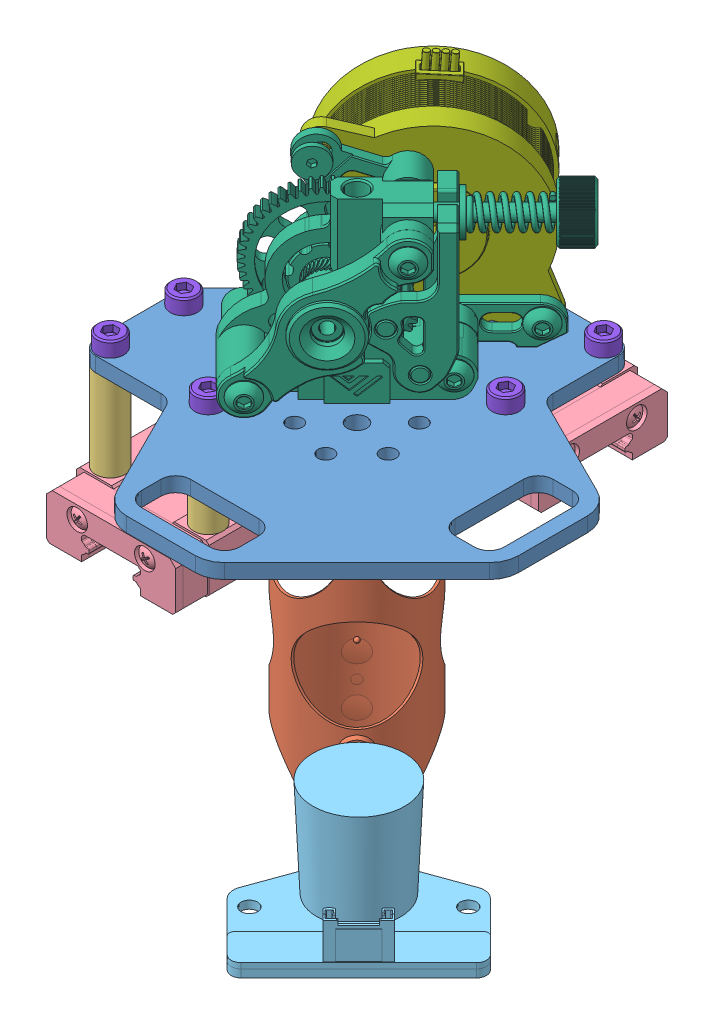
SolidWorks assembly ASM_Printhead_V1, configuration Default. Lengths in mm.
Overall size (87.58 123.94 98.13).
20 component instances, 8 part files, 39 mates.
Components (placement in the parent):
- PRT_Main_Plate_V1-1: PRT_Main_Plate_V1 [Default] at (19.5589 25.187 46.8985) size (81.5 3 81.5)
- PRT_Chube_Integration_V2-1: PRT_Chube_Integration_V2 [Default] at (-4.1383 -257.0883 22.8287) x (0.707107 0 -0.707107) z (0 1 0) size (26.81 27.92 66)
- PRT_M3x18_Standoff_V1-2: PRT_M3x18_Standoff_V1 [Default] at (-18.9411 7.187 58.7485) size (6 18 6)
- PRT_M3x18_Standoff_V1-3: PRT_M3x18_Standoff_V1 [Default] at (1.0589 7.187 58.7485) size (6 18 6)
- PRT_M3x18_Standoff_V1-4: PRT_M3x18_Standoff_V1 [Default] at (1.0589 7.187 43.7485) size (6 18 6)
- PRT_M3x18_Standoff_V1-5: PRT_M3x18_Standoff_V1 [Default] at (-18.9411 7.187 43.7485) size (6 18 6)
- PRT_MGN12C_Carriage-1: PRT_MGN12C_Carriage [Default] at (-8.9411 -0.313 51.2485) size (27 10 37.07)
- PRT_MGN12C_Carriage-2: PRT_MGN12C_Carriage [Default] at (23.9089 17.687 18.3985) x (0 0 -1) z (1 0 0) size (27 10 37.07)
- PRT_Beacon_RevH_Assm_Normal-1: PRT_Beacon_RevH_Assm_Normal [Default] at (38.27 -36.4022 65.237) x (0.707107 0 -0.707107) z (0 1 0) size (38 28.37 24.21)
- ASM_MA_Extruder_V1-1: ASM_MA_Extruder_V1 [Default] at (-20.6578 21.9691 29.4732) x (0.707107 0 -0.707107) z (0.707107 0 0.707107) size (62.49 57.22 45.42)
  - PRT_MA_VZ_Hextrudort-2: PRT_MA_VZ_Hextrudort [Default] at (16.116 12.2179 40.659) x (1 0 0) z (0 1 0) size (55.08 29 38.4)
  - PRT_MA_LDO_20mm_Nema14-1: PRT_MA_LDO_20mm_Nema14 [Default] at (-5.0462 48.6582 8.2878) x (-0.88148 0.472221 -0.000518) z (0.000441 -0.000274 -1) size (48.79 38.77 26.01)
- socket head cap screw_am-1: socket head cap screw_am [B18.3.1M - 3 x 0.5 x 25 Hex SHCS -- 18NHX] at (1.0589 31.187 58.7485) x (0 -1 0) z (0 0 1) size (28 5.5 5.5)
- socket head cap screw_am-2: socket head cap screw_am [B18.3.1M - 3 x 0.5 x 25 Hex SHCS -- 18NHX] at (-18.9411 31.187 58.7485) x (0 -1 0) z (0 0 1) size (28 5.5 5.5)
- socket head cap screw_am-3: socket head cap screw_am [B18.3.1M - 3 x 0.5 x 25 Hex SHCS -- 18NHX] at (-18.9411 31.187 43.7485) x (0 -1 0) z (0 0 1) size (28 5.5 5.5)
- socket head cap screw_am-4: socket head cap screw_am [B18.3.1M - 3 x 0.5 x 25 Hex SHCS -- 18NHX] at (1.0589 31.187 43.7485) x (0 -1 0) z (0 0 1) size (28 5.5 5.5)
- socket head cap screw_am-6: socket head cap screw_am [B18.3.1M - 3 x 0.5 x 6 Hex SHCS -- 6NHX] at (31.4089 31.187 8.3985) x (0 -1 0) z (0 0 1) size (9 5.5 5.5)
- socket head cap screw_am-7: socket head cap screw_am [B18.3.1M - 3 x 0.5 x 6 Hex SHCS -- 6NHX] at (31.4089 31.187 28.3985) x (0 -1 0) z (0 0 1) size (9 5.5 5.5)
- socket head cap screw_am-8: socket head cap screw_am [B18.3.1M - 3 x 0.5 x 6 Hex SHCS -- 6NHX] at (16.4089 31.187 28.3985) x (0 -1 0) z (0 0 1) size (9 5.5 5.5)
- socket head cap screw_am-9: socket head cap screw_am [B18.3.1M - 3 x 0.5 x 6 Hex SHCS -- 6NHX] at (16.4089 31.187 8.3985) x (0 -1 0) z (0 0 1) size (9 5.5 5.5)
Mates (geometry in assembly coordinates):
- Concentric1: concentric anti-aligned: cylinder of PRT_Main_Plate_V1-1 through (19.5589 28.187 46.8985) axis (0 1 0) radius 2; cylinder of PRT_Chube_Integration_V2-1 through (19.5589 25.187 46.8985) axis (0 -1 0) radius 2.05
- Coincident1: coincident anti-aligned: plane of PRT_Main_Plate_V1-1 through (19.5589 25.187 46.8985) normal (0 -1 0); plane of PRT_Chube_Integration_V2-1 through (22.0338 25.187 44.4236) normal (0 1 0)
- Concentric3: concentric anti-aligned: cylinder of PRT_Main_Plate_V1-1 through (13.195 28.187 53.2625) axis (0 1 0) radius 1.6; cylinder of PRT_Chube_Integration_V2-1 through (13.195 25.187 53.2625) axis (0 -1 0) radius 1.5
- Concentric41: concentric anti-aligned: cylinder of PRT_Main_Plate_V1-1 through (-18.9411 28.187 58.7485) axis (0 1 0) radius 1.6; cylinder of PRT_M3x18_Standoff_V1-2 through (-18.9411 25.187 58.7485) axis (0 -1 0) radius 3
- Coincident21: coincident anti-aligned: plane of PRT_Main_Plate_V1-1 through (19.5589 25.187 46.8985) normal (0 -1 0); plane of PRT_M3x18_Standoff_V1-2 through (-18.9411 25.187 58.7485) normal (0 1 0)
- Concentric51: concentric anti-aligned: cylinder of PRT_Main_Plate_V1-1 through (1.0589 28.187 58.7485) axis (0 1 0) radius 1.6; cylinder of PRT_M3x18_Standoff_V1-3 through (1.0589 25.187 58.7485) axis (0 -1 0) radius 3
- Coincident31: coincident anti-aligned: plane of PRT_Main_Plate_V1-1 through (19.5589 25.187 46.8985) normal (0 -1 0); plane of PRT_M3x18_Standoff_V1-3 through (1.0589 25.187 58.7485) normal (0 1 0)
- Concentric61: concentric anti-aligned: cylinder of PRT_Main_Plate_V1-1 through (1.0589 28.187 43.7485) axis (0 1 0) radius 1.6; cylinder of PRT_M3x18_Standoff_V1-4 through (1.0589 25.187 43.7485) axis (0 -1 0) radius 3
- Coincident41: coincident anti-aligned: plane of PRT_Main_Plate_V1-1 through (19.5589 25.187 46.8985) normal (0 -1 0); plane of PRT_M3x18_Standoff_V1-4 through (1.0589 25.187 43.7485) normal (0 1 0)
- Concentric71: concentric anti-aligned: cylinder of PRT_Main_Plate_V1-1 through (-18.9411 28.187 43.7485) axis (0 1 0) radius 1.6; cylinder of PRT_M3x18_Standoff_V1-5 through (-18.9411 25.187 43.7485) axis (0 -1 0) radius 3
- Coincident51: coincident anti-aligned: plane of PRT_Main_Plate_V1-1 through (19.5589 25.187 46.8985) normal (0 -1 0); plane of PRT_M3x18_Standoff_V1-5 through (-18.9411 25.187 43.7485) normal (0 1 0)
- Concentric8: concentric anti-aligned: cylinder of PRT_M3x18_Standoff_V1-4 through (1.0589 25.187 43.7485) axis (0 -1 0) radius 3; cylinder of PRT_MGN12C_Carriage-1 through (1.0589 7.187 43.7485) axis (0 1 0) radius 1.5
- Concentric9: concentric anti-aligned: cylinder of PRT_M3x18_Standoff_V1-2 through (-18.9411 25.187 58.7485) axis (0 -1 0) radius 3; cylinder of PRT_MGN12C_Carriage-1 through (-18.9411 7.187 58.7485) axis (0 1 0) radius 1.5
- Coincident6: coincident anti-aligned: plane of PRT_M3x18_Standoff_V1-2 through (-18.9411 7.187 58.7485) normal (0 -1 0); plane of PRT_MGN12C_Carriage-1 through (-15.3411 7.187 62.0985) normal (0 1 0)
- Concentric10: concentric aligned: cylinder of PRT_Main_Plate_V1-1 through (31.4089 28.187 28.3985) axis (0 1 0) radius 1.6; cylinder of PRT_MGN12C_Carriage-2 through (31.4089 25.187 28.3985) axis (0 1 0) radius 1.5
- Concentric11: concentric aligned: cylinder of PRT_Main_Plate_V1-1 through (16.4089 28.187 8.3985) axis (0 1 0) radius 1.6; cylinder of PRT_MGN12C_Carriage-2 through (16.4089 25.187 8.3985) axis (0 1 0) radius 1.5
- Coincident7: coincident anti-aligned: plane of PRT_Main_Plate_V1-1 through (19.5589 25.187 46.8985) normal (0 -1 0); plane of PRT_MGN12C_Carriage-2 through (34.7589 25.187 5.4985) normal (0 1 0)
- Concentric12: concentric aligned: cylinder of PRT_Main_Plate_V1-1 through (1.0589 28.187 58.7485) axis (0 1 0) radius 1.6; cylinder of socket head cap screw_am-1 through (1.0589 62.937 58.7485) axis (0 1 0) radius 2.75
- Coincident8: coincident anti-aligned: plane of PRT_Main_Plate_V1-1 through (19.5589 28.187 46.8985) normal (0 1 0); plane of socket head cap screw_am-1 through (3.8089 28.187 58.7485) normal (0 -1 0)
- Concentric13: concentric aligned: cylinder of PRT_Main_Plate_V1-1 through (-18.9411 28.187 58.7485) axis (0 1 0) radius 1.6; cylinder of socket head cap screw_am-2 through (-18.9411 62.937 58.7485) axis (0 1 0) radius 2.75
- Coincident9: coincident anti-aligned: plane of PRT_Main_Plate_V1-1 through (19.5589 28.187 46.8985) normal (0 1 0); plane of socket head cap screw_am-2 through (-16.1911 28.187 58.7485) normal (0 -1 0)
- Concentric14: concentric aligned: cylinder of PRT_Main_Plate_V1-1 through (-18.9411 28.187 43.7485) axis (0 1 0) radius 1.6; cylinder of socket head cap screw_am-3 through (-18.9411 62.937 43.7485) axis (0 1 0) radius 2.75
- Coincident10: coincident anti-aligned: plane of PRT_Main_Plate_V1-1 through (19.5589 28.187 46.8985) normal (0 1 0); plane of socket head cap screw_am-3 through (-16.1911 28.187 43.7485) normal (0 -1 0)
- Concentric15: concentric aligned: cylinder of PRT_Main_Plate_V1-1 through (1.0589 28.187 43.7485) axis (0 1 0) radius 1.6; cylinder of socket head cap screw_am-4 through (1.0589 62.937 43.7485) axis (0 1 0) radius 2.75
- Coincident11: coincident anti-aligned: plane of PRT_Main_Plate_V1-1 through (19.5589 28.187 46.8985) normal (0 1 0); plane of socket head cap screw_am-4 through (3.8089 28.187 43.7485) normal (0 -1 0)
- Concentric17: concentric aligned: cylinder of PRT_Main_Plate_V1-1 through (31.4089 28.187 8.3985) axis (0 1 0) radius 1.6; cylinder of socket head cap screw_am-6 through (31.4089 62.937 8.3985) axis (0 1 0) radius 2.75
- Coincident13: coincident anti-aligned: plane of PRT_Main_Plate_V1-1 through (19.5589 28.187 46.8985) normal (0 1 0); plane of socket head cap screw_am-6 through (34.1589 28.187 8.3985) normal (0 -1 0)
- Concentric18: concentric aligned: cylinder of PRT_Main_Plate_V1-1 through (31.4089 28.187 28.3985) axis (0 1 0) radius 1.6; cylinder of socket head cap screw_am-7 through (31.4089 62.937 28.3985) axis (0 1 0) radius 2.75
- Coincident14: coincident anti-aligned: plane of PRT_Main_Plate_V1-1 through (19.5589 28.187 46.8985) normal (0 1 0); plane of socket head cap screw_am-7 through (34.1589 28.187 28.3985) normal (0 -1 0)
- Concentric19: concentric aligned: cylinder of PRT_Main_Plate_V1-1 through (16.4089 28.187 28.3985) axis (0 1 0) radius 1.6; cylinder of socket head cap screw_am-8 through (16.4089 62.937 28.3985) axis (0 1 0) radius 2.75
- Coincident15: coincident anti-aligned: plane of PRT_Main_Plate_V1-1 through (19.5589 28.187 46.8985) normal (0 1 0); plane of socket head cap screw_am-8 through (19.1589 28.187 28.3985) normal (0 -1 0)
- Concentric20: concentric aligned: cylinder of PRT_Main_Plate_V1-1 through (16.4089 28.187 8.3985) axis (0 1 0) radius 1.6; cylinder of socket head cap screw_am-9 through (16.4089 62.937 8.3985) axis (0 1 0) radius 2.75
- Coincident16: coincident anti-aligned: plane of PRT_Main_Plate_V1-1 through (19.5589 28.187 46.8985) normal (0 1 0); plane of socket head cap screw_am-9 through (19.1589 28.187 8.3985) normal (0 -1 0)
- Distance2: distance = 4.8 mm aligned: plane of PRT_Beacon_RevH_Assm_Normal-1 through (38.27 -40.613 65.237) normal (0 -1 0); plane of PRT_Chube_Integration_V2-1 through (19.5589 -35.813 46.8985) normal (0 -1 0)
- Distance3: distance = 17.7 mm: point of PRT_Beacon_RevH_Assm_Normal-1; cylinder of PRT_Chube_Integration_V2-1 through (19.5589 -34.813 46.8985) axis (0 1 0) radius 12.7
- Coincident19: coincident aligned: plane of PRT_Chube_Integration_V2-1 through (-4.1383 -257.0883 22.8287) normal (0.707107 0 -0.707107); plane of PRT_Beacon_RevH_Assm_Normal-1 through (38.27 -36.4022 65.237) normal (0.707107 0 -0.707107)
- Concentric72: concentric anti-aligned: cylinder of PRT_Main_Plate_V1-1 through (19.5589 28.187 46.8985) axis (0 1 0) radius 2; cylinder of ASM_MA_Extruder_V1-1/PRT_MA_VZ_Hextrudort-2 through (19.5589 42.187 46.8985) axis (0 -1 0) radius 2.05
- Distance4: distance = 6 mm anti-aligned: plane of ASM_MA_Extruder_V1-1/PRT_MA_VZ_Hextrudort-2 through (10.9405 34.187 66.4771) normal (0 -1 0); plane of PRT_Main_Plate_V1-1 through (19.5589 28.187 46.8985) normal (0 1 0)
- Parallel1: parallel aligned: plane of PRT_Main_Plate_V1-1 through (-21.9411 28.187 40.7485) normal (-0.707107 0 -0.707107); plane of ASM_MA_Extruder_V1-1/PRT_MA_LDO_20mm_Nema14-1 through (4.2129 53.4752 16.0704) normal (-0.707107 0 -0.707107)
